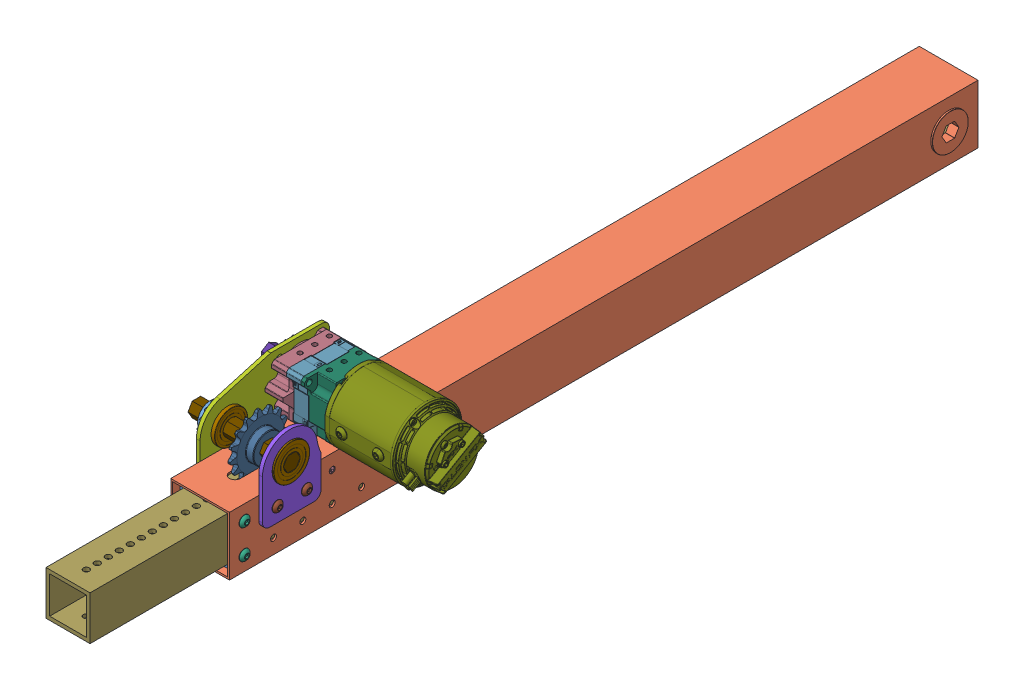
SolidWorks assembly GOOD Telescoping+Powered+Arm+ASM, configuration Default. Lengths in mm.
Overall size (167.89 110.27 901.7).
57 component instances, 23 part files, 25 mates.
Components (placement in the parent):
- Telescoping+Powered+Arm+ASM.stp-1: Telescoping+Powered+Arm+ASM.stp [Default] at origin size (82.02 101.6 1168.4)
  - 2x2tube ASM.stp-1: 2x2tube ASM.stp [Default] at origin size (55.93 50.8 914.4)
    - Slider_Blocks.stp-1: Slider_Blocks.stp [Default] at origin size (17.4 47.5 12.7)
      - Slider_Blocks_4.stp-1: Slider_Blocks_4.stp [Default] at (-0.0635 1254.125 -781.05) x (0 1 0) z (-1 0 0) size (47.5 12.7 17.4)
    - Slider_Blocks_1.stp-1: Slider_Blocks_1.stp [Default] at origin size (17.4 47.5 12.7)
      - Slider_Blocks_4.stp-1: Slider_Blocks_4.stp [Default] at (-0.0635 1254.125 -908.05) x (0 1 0) z (-1 0 0) size (47.5 12.7 17.4)
    - Slider_Blocks_2.stp-1: Slider_Blocks_2.stp [Default] at origin size (17.4 47.5 12.7)
      - Slider_Blocks_4.stp-1: Slider_Blocks_4.stp [Default] at (0.0635 -1254.125 -781.05) x (0 -1 0) z (1 0 0) size (47.5 12.7 17.4)
    - Slider_Blocks_3.stp-1: Slider_Blocks_3.stp [Default] at origin size (17.4 47.5 12.7)
      - Slider_Blocks_4.stp-1: Slider_Blocks_4.stp [Default] at (0.0635 -1254.125 -908.05) x (0 -1 0) z (1 0 0) size (47.5 12.7 17.4)
    - 2x2 long Stick.stp-1: 2x2 long Stick.stp [Default] at origin size (50.8 50.8 914.4)
    - 95185A190_Zinc-Plated Steel Press-Fit Nut for Sheet Metal.stp-1: 95185A190_Zinc-Plated Steel Press-Fit Nut for Sheet Metal.stp [Default] at (-21.5265 12.7 -38.1) x (0 0 -1) z (1 0 0) size (8.64 8.64 3.71)
    - 95185A190_Zinc-Plated Steel Press-Fit Nut for Sheet Metal.stp-2: 95185A190_Zinc-Plated Steel Press-Fit Nut for Sheet Metal.stp [Default] at (-21.5265 12.7 -63.5) x (0 0 -1) z (1 0 0) size (8.64 8.64 3.71)
    - 95185A190_Zinc-Plated Steel Press-Fit Nut for Sheet Metal.stp-3: 95185A190_Zinc-Plated Steel Press-Fit Nut for Sheet Metal.stp [Default] at (-21.5265 12.7 -88.9) x (0 0 -1) z (1 0 0) size (8.64 8.64 3.71)
    - 95185A190_Zinc-Plated Steel Press-Fit Nut for Sheet Metal.stp-4: 95185A190_Zinc-Plated Steel Press-Fit Nut for Sheet Metal.stp [Default] at (-21.5265 12.7 -114.3) x (0 0 -1) z (1 0 0) size (8.64 8.64 3.71)
    - 95185A190_Zinc-Plated Steel Press-Fit Nut for Sheet Metal(Mirror).stp-1: 95185A190_Zinc-Plated Steel Press-Fit Nut for Sheet Metal(Mirror).stp [Default] at (21.5265 12.7 -38.1) x (0 0 -1) z (1 0 0) size (8.64 8.64 3.71)
    - 95185A190_Zinc-Plated Steel Press-Fit Nut for Sheet Metal(Mirror).stp-2: 95185A190_Zinc-Plated Steel Press-Fit Nut for Sheet Metal(Mirror).stp [Default] at (21.5265 12.7 -63.5) x (0 0 -1) z (1 0 0) size (8.64 8.64 3.71)
    - 95185A190_Zinc-Plated Steel Press-Fit Nut for Sheet Metal(Mirror).stp-3: 95185A190_Zinc-Plated Steel Press-Fit Nut for Sheet Metal(Mirror).stp [Default] at (21.5265 12.7 -88.9) x (0 0 -1) z (1 0 0) size (8.64 8.64 3.71)
    - 95185A190_Zinc-Plated Steel Press-Fit Nut for Sheet Metal(Mirror).stp-4: 95185A190_Zinc-Plated Steel Press-Fit Nut for Sheet Metal(Mirror).stp [Default] at (21.5265 12.7 -114.3) x (0 0 -1) z (1 0 0) size (8.64 8.64 3.71)
    - 91255A025_Button Head Hex Drive Screw.stp-1: 91255A025_Button Head Hex Drive Screw.stp [Default] at (-24.3014 -12.7 -12.7) x (0 0 1) z (-1 0 0) size (9.16 9.16 7.33)
    - 91255A025_Button Head Hex Drive Screw.stp-2: 91255A025_Button Head Hex Drive Screw.stp [Default] at (-24.3014 12.7 -12.7) x (0 0 1) z (-1 0 0) size (9.16 9.16 7.33)
    - 91255A025_Button Head Hex Drive Screw.stp-3: 91255A025_Button Head Hex Drive Screw.stp [Default] at (-24.3014 12.7 -139.7) x (0 0 1) z (-1 0 0) size (9.16 9.16 7.33)
    - 91255A025_Button Head Hex Drive Screw.stp-4: 91255A025_Button Head Hex Drive Screw.stp [Default] at (-24.3014 -12.7 -139.7) x (0 0 1) z (-1 0 0) size (9.16 9.16 7.33)
    - 91255A025_Button Head Hex Drive Screw(Mirror).stp-1: 91255A025_Button Head Hex Drive Screw(Mirror).stp [Default] at (24.3014 -12.7 -12.7) x (0 0 1) z (-1 0 0) size (9.16 9.16 7.33)
    - 91255A025_Button Head Hex Drive Screw(Mirror).stp-2: 91255A025_Button Head Hex Drive Screw(Mirror).stp [Default] at (24.3014 12.7 -12.7) x (0 0 1) z (-1 0 0) size (9.16 9.16 7.33)
    - 91255A025_Button Head Hex Drive Screw(Mirror).stp-3: 91255A025_Button Head Hex Drive Screw(Mirror).stp [Default] at (24.3014 12.7 -139.7) x (0 0 1) z (-1 0 0) size (9.16 9.16 7.33)
    - 91255A025_Button Head Hex Drive Screw(Mirror).stp-4: 91255A025_Button Head Hex Drive Screw(Mirror).stp [Default] at (24.3014 -12.7 -139.7) x (0 0 1) z (-1 0 0) size (9.16 9.16 7.33)
  - gear box.stp-1: gear box.stp [Default] at (-25.4 12.7 -38.1) x (0 -1 0) z (1 0 0) size (76.2 113.36 82.02)
    - Selft_drive_Guesset.stp-1: Selft_drive_Guesset.stp [Default] at (12.7 -38.1 25.4) x (0 0 1) z (0 -1 0) size (3.18 76.2 111.91)
      - Selft_drive_Guesset_1.stp-1: Selft_drive_Guesset_1.stp [Default] at (0 -1254.125 -508) x (0 -1 0) z (1 0 0) size (76.2 111.91 3.18)
    - Selfie_drive_guesset_small.stp-1: Selfie_drive_guesset_small.stp [Default] at (12.7 -38.1 25.4) x (0 0 1) z (0 -1 0) size (3.18 64.58 50.8)
      - Selfie_drive_guesset_small_1.stp-1: Selfie_drive_guesset_small_1.stp [Default] at (50.8 -1254.125 -508) x (0 -1 0) z (1 0 0) size (64.58 50.8 3.17)
    - Ball Bearing.stp-1: Ball Bearing.stp [Default] at (-28.067 11.1125 -0.7937) x (1 0 0) z (0 0 -1) size (31.12 31.12 7.94)
    - Ball Bearing.stp-2: Ball Bearing.stp [Default] at (-28.067 11.1125 51.5938) size (31.12 31.12 7.94)
    - hex shaft.stp-1: hex shaft.stp [Default] at (-28.067 11.1125 -388.9375) size (13.74 12.75 73.03) (hidden)
    - 93286A013_Aluminum Washer.stp-1: 93286A013_Aluminum Washer.stp [Default] at (-28.067 11.1125 -5.334) x (0 0 1) z (-1 0 0) size (1.14 17.48 17.48) (hidden)
    - 93286A013_Aluminum Washer.stp-2: 93286A013_Aluminum Washer.stp [Default] at (-28.067 11.1125 68.834) x (0 0 -1) z (1 0 0) size (1.14 17.48 17.48) (hidden)
    - 91255A535_Button Head Hex Drive Screw.stp-1: 91255A535_Button Head Hex Drive Screw.stp [Default] at (-28.067 11.1125 -2.8194) x (1 0 0) z (0 0 -1) size (11.09 11.09 12.88) (hidden)
    - 91255A535_Button Head Hex Drive Screw.stp-2: 91255A535_Button Head Hex Drive Screw.stp [Default] at (-28.067 11.1125 66.3194) size (11.09 11.09 12.88) (hidden)
    - 15 Tooth Sprocket.stp-1: 15 Tooth Sprocket.stp [Default] at (-28.067 11.1125 26.397) size (50.31 50.58 10.68)
    - 91255A262_Button Head Hex Drive Screw.stp-1: 91255A262_Button Head Hex Drive Screw.stp [Default] at (0 76.2 -0.489) x (1 0 0) z (0 0 -1) size (9.16 9.16 10.5)
    - 91255A262_Button Head Hex Drive Screw.stp-2: 91255A262_Button Head Hex Drive Screw.stp [Default] at (0 50.8 -0.489) x (1 0 0) z (0 0 -1) size (9.16 9.16 10.5)
    - 91255A262_Button Head Hex Drive Screw.stp-3: 91255A262_Button Head Hex Drive Screw.stp [Default] at (0 25.4 51.2889) size (9.16 9.16 10.5)
    - 91255A262_Button Head Hex Drive Screw.stp-4: 91255A262_Button Head Hex Drive Screw.stp [Default] at (0 0 -0.489) x (1 0 0) z (0 0 -1) size (9.16 9.16 10.5)
    - 91255A262_Button Head Hex Drive Screw.stp-5: 91255A262_Button Head Hex Drive Screw.stp [Default] at (0 25.4 -0.489) x (1 0 0) z (0 0 -1) size (9.16 9.16 10.5)
    - 91255A262_Button Head Hex Drive Screw.stp-6: 91255A262_Button Head Hex Drive Screw.stp [Default] at (0 0 51.2889) size (9.16 9.16 10.5)
  - 1.5 slide tube.stp-1: 1.5 slide tube.stp [Default] at (-19.05 -19.05 -914.4) size (38.1 38.1 1168.4)
- gearbox 1-1: gearbox 1 [Default] at (-15.875 50.8 -111.9149) x (-1 0 0) z (0 0 -1) size (23.2 50.8 61.92)
- gearbox 2-2: gearbox 2 [Default] at (0 50.8 -111.9149) x (0 0 1) z (-1 0 0) size (61.91 50.8 16.85)
- gearbox 3-1: gearbox 3 [Default] at (15.875 50.8 -111.9149) x (0 0 1) z (-1 0 0) size (61.91 50.8 19.05)
- Falcon 500, Powered by Talon FX (Rev 3) (217-6515).step-1: Falcon 500, Powered by Talon FX (Rev 3) (217-6515).step [Default] at (86.15 50.8 -111.9149) x (0 0 1) z (-1 0 0) size (62.05 60 125.3)
- 1in hex axle-1: 1in hex axle [Default] at (-52.3875 50.8003 -111.9276) x (0 -0.481071 -0.876682) z (1 0 0) size (14.66 12.7 38.1)
- 3.25in hex axle-1: 3.25in hex axle [Default] at (-52.3875 40.7543 -49.2345) x (0 -0.866025 0.5) z (1 0 0) size (14.66 12.7 82.55)
- 18 tooth sprocket.step-1: 18 tooth sprocket.step [Default] at (-34.29 50.8025 -112.0292) x (0 -0.481071 -0.876682) z (1 0 0) size (39.38 39.82 10.29)
- 18 tooth sprocket.step-2: 18 tooth sprocket.step [Default] at (-31.5595 40.8051 -49.1465) x (0 0 1) z (-1 0 0) size (39.38 39.82 10.29)
- am-2986 FR8ZZ Hex Bearing.step-1: am-2986 FR8ZZ Hex Bearing.step [Default] at (18.9967 0 -622.3) x (0 0 -1) z (1 0 0) size (31.12 31.12 7.93)
- am-2986 FR8ZZ Hex Bearing.step-2: am-2986 FR8ZZ Hex Bearing.step [Default] at (-18.9967 0 -622.3) x (0 0 1) z (-1 0 0) size (31.12 31.12 7.93)
Mates (geometry in assembly coordinates):
- Concentric1: concentric anti-aligned: circle of Telescoping+Powered+Arm+ASM.stp-1/gear box.stp-1/Selft_drive_Guesset.stp-1/Selft_drive_Guesset_1.stp-1; circle of gearbox 1-1
- Concentric2: concentric aligned: cylinder of Telescoping+Powered+Arm+ASM.stp-1/gear box.stp-1/Selft_drive_Guesset.stp-1/Selft_drive_Guesset_1.stp-1 through (-25.4 32.8395 -93.9544) axis (-1 0 0) radius 2.5797; circle of gearbox 1-1
- Coincident1: coincident anti-aligned: plane of Telescoping+Powered+Arm+ASM.stp-1/gear box.stp-1/Selft_drive_Guesset.stp-1/Selft_drive_Guesset_1.stp-1 through (-25.4 37.7767 -83.6718) normal (1 0 0); plane of gearbox 1-1 through (-25.4 50.8 -111.9149) normal (-1 0 0)
- Concentric8: concentric anti-aligned: cylinder of gearbox 1-1 through (-28.7329 50.8 -111.9149) axis (1 0 0) radius 5.5563; circle of gearbox 2-2
- Coincident5: coincident anti-aligned: plane of gearbox 1-1 through (-6.35 50.8 -111.9149) normal (1 0 0); plane of gearbox 2-2 through (-6.35 50.8 -111.9149) normal (-1 0 0)
- Coincident6: coincident anti-aligned: plane of gearbox 2-2 through (6.35 50.8 -111.9149) normal (1 0 0); plane of gearbox 3-1 through (6.35 50.8 -111.9149) normal (-1 0 0)
- Coincident7: coincident aligned: plane of gearbox 2-2 through (-6.35 67.564 -137.3149) normal (0 0.707107 -0.707107); plane of gearbox 3-1 through (6.35 71.882 -132.9969) normal (0 0.707107 -0.707107)
- Coincident8: coincident aligned: plane of gearbox 2-2 through (-6.35 25.4 -137.3149) normal (0 0 -1); plane of gearbox 3-1 through (6.35 50.8 -137.3149) normal (0 0 -1)
- Concentric9: concentric anti-aligned: cylinder of gearbox 3-1 through (6.35 50.8 -111.9149) axis (1 0 0) radius 9.5504; circle of Falcon 500, Powered by Talon FX (Rev 3) (217-6515).step-1
- Coincident9: coincident anti-aligned: plane of gearbox 3-1 through (25.4 50.8 -111.9149) normal (1 0 0); plane of Falcon 500, Powered by Talon FX (Rev 3) (217-6515).step-1 through (25.4 42.5511 -116.6774) normal (-1 0 0)
- Coincident10: coincident anti-aligned: plane of gearbox 1-1 through (-14.2875 50.8 -111.9149) normal (-1 0 0); plane of 1in hex axle-1 through (-14.2875 50.8003 -111.9276) normal (1 0 0)
- Coincident11: coincident: plane of gearbox 1-1 through (-14.2875 47.2691 -118.3494) normal (0 0.85496 0.518693); line of 1in hex axle-1 through (-14.2875 43.4697 -112.0868) axis (0 0.518693 -0.85496)
- Coincident12: coincident anti-aligned: plane of gearbox 1-1 through (-14.2875 58.1379 -111.7555) normal (0 -0.876682 0.481071); plane of 1in hex axle-1 through (-14.2875 54.6035 -118.1964) normal (0 0.876682 -0.481071)
- Coincident14: coincident aligned: plane of Telescoping+Powered+Arm+ASM.stp-1/gear box.stp-1/Ball Bearing.stp-2 through (30.1625 40.767 -64.7725) normal (1 0 0); plane of 3.25in hex axle-1 through (30.1625 40.7543 -49.2345) normal (1 0 0)
- Coincident15: coincident anti-aligned: plane of Telescoping+Powered+Arm+ASM.stp-1/gear box.stp-1/15 Tooth Sprocket.stp-1 through (9.526 40.767 -56.5595) normal (0 -0.5 0.866025); plane of 3.25in hex axle-1 through (30.1625 40.7543 -56.5668) normal (0 0.5 -0.866025)
- Coincident16: coincident anti-aligned: plane of Telescoping+Powered+Arm+ASM.stp-1/gear box.stp-1/15 Tooth Sprocket.stp-1 through (9.526 34.4043 -45.539) normal (0 1 0); plane of 3.25in hex axle-1 through (30.1625 34.4043 -45.5683) normal (0 -1 0)
- Coincident22: coincident anti-aligned: plane of Telescoping+Powered+Arm+ASM.stp-1/gear box.stp-1/Ball Bearing.stp-1 through (-30.1625 40.767 -39.6105) normal (-1 0 0); plane of 18 tooth sprocket.step-2 through (-30.1625 24.0688 -49.1465) normal (1 0 0)
- Coincident23: coincident anti-aligned: plane of 3.25in hex axle-1 through (30.1625 34.4043 -45.5683) normal (0 -1 0); plane of 18 tooth sprocket.step-2 through (-30.1625 34.4043 -52.842) normal (0 1 0)
- Coincident24: coincident anti-aligned: plane of 3.25in hex axle-1 through (30.1625 40.7543 -56.5668) normal (0 0.5 -0.866025); plane of 18 tooth sprocket.step-2 through (-30.1625 47.2059 -52.842) normal (0 -0.5 0.866025)
- Concentric11: concentric: cylinder of Telescoping+Powered+Arm+ASM.stp-1/2x2tube ASM.stp-1/2x2 long Stick.stp-1 through (-20.828 0 -413.7836) axis (-1 0 0) radius 14.2875; cylinder of am-2986 FR8ZZ Hex Bearing (1).step-2 through (-26.924 0 -413.7836) axis (1 0 0) radius 14.2875
- Coincident26: coincident anti-aligned: plane of Telescoping+Powered+Arm+ASM.stp-1/2x2tube ASM.stp-1/2x2 long Stick.stp-1 through (-25.4 -25.4 0) normal (-1 0 0); plane of am-2986 FR8ZZ Hex Bearing (1).step-2 through (-25.4 -0.0664 -399.8138) normal (1 0 0)
- Concentric12: concentric anti-aligned: cylinder of Telescoping+Powered+Arm+ASM.stp-1/2x2tube ASM.stp-1/2x2 long Stick.stp-1 through (20.32 0 -622.3) axis (1 0 0) radius 14.2875; cylinder of am-2986 FR8ZZ Hex Bearing.step-1 through (26.924 0 -622.3) axis (-1 0 0) radius 14.2875
- Coincident27: coincident anti-aligned: plane of Telescoping+Powered+Arm+ASM.stp-1/2x2tube ASM.stp-1/2x2 long Stick.stp-1 through (25.4 25.4 0) normal (1 0 0); plane of am-2986 FR8ZZ Hex Bearing.step-1 through (25.4 0 -636.27) normal (-1 0 0)
- Concentric13: concentric anti-aligned: cylinder of Telescoping+Powered+Arm+ASM.stp-1/2x2tube ASM.stp-1/2x2 long Stick.stp-1 through (-20.828 0 -622.3) axis (-1 0 0) radius 14.2875; cylinder of am-2986 FR8ZZ Hex Bearing.step-2 through (-26.924 0 -622.3) axis (1 0 0) radius 14.2875
- Coincident28: coincident anti-aligned: plane of Telescoping+Powered+Arm+ASM.stp-1/2x2tube ASM.stp-1/2x2 long Stick.stp-1 through (-25.4 -25.4 0) normal (-1 0 0); plane of am-2986 FR8ZZ Hex Bearing.step-2 through (-25.4 0 -608.33) normal (1 0 0)
